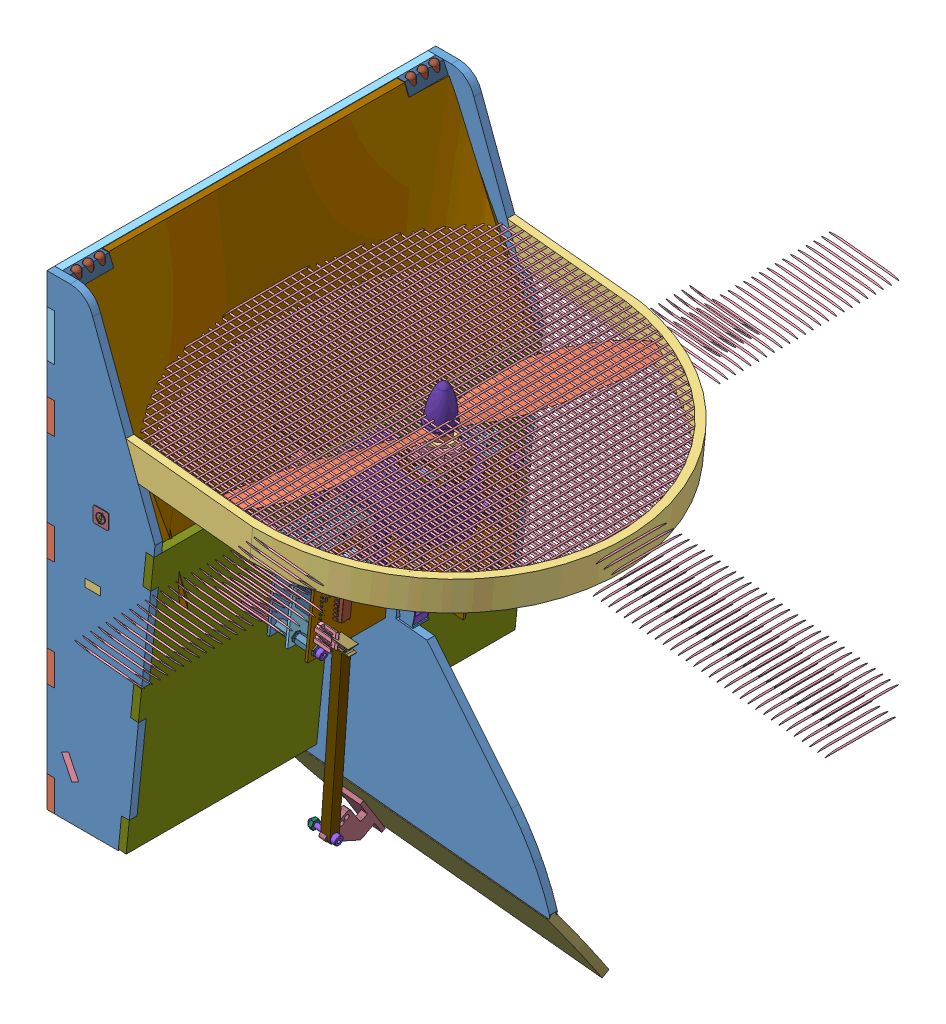
SolidWorks assembly AssTotaleSimu7, configuration Défaut. Lengths in mm. (continued)
Components (placement in the parent): (continued)
- AssStructSimu-1: AssStructSimu [Défaut] at (-125.7658 -1.8483 624.6548) x (1 0 0) z (0 0 -1) size (253.25 324.59 251.6) (continued)
  - AssProtec-1: AssProtec [Défaut] at (86.6746 190.4649 284.6351) x (0 0 -1) z (0.101852 -0.9948 0) size (250 237.46 20) (continued)
    - AssGrillage-2: AssGrillage [Défaut] at (339.6086 -132.5428 241.6839) x (0 0 1) z (-1 0 0) size (2.02 237.05 250) (continued)
      - barreau-208: barreau [Défaut] at (-0.1839 -1.5314 233.7823) x (0.998922 0 0.04641) z (0 1 0) size (1 1 400)
      - barreau-209: barreau [Défaut] at (-0.1839 -1.5314 228.7823) x (0.998922 0 0.04641) z (0 1 0) size (1 1 400)
      - barreau-210: barreau [Défaut] at (-0.1839 -1.5314 223.7823) x (0.998922 0 0.04641) z (0 1 0) size (1 1 400)
      - barreau-211: barreau [Défaut] at (-0.1839 -1.5314 218.7823) x (0.998922 0 0.04641) z (0 1 0) size (1 1 400)
      - barreau-212: barreau [Défaut] at (-0.1839 -1.5314 213.7823) x (0.998922 0 0.04641) z (0 1 0) size (1 1 400)
      - barreau-213: barreau [Défaut] at (-0.1839 -1.5314 208.7823) x (0.998922 0 0.04641) z (0 1 0) size (1 1 400)
      - barreau-214: barreau [Défaut] at (-0.1839 -1.5314 203.7823) x (0.998922 0 0.04641) z (0 1 0) size (1 1 400)
  - AssCarte-1: AssCarte [Défaut] at (38.0121 147.1029 290.772) x (-0.101852 0.9948 0) z (0.9948 0.101852 0) size (66.52 130.57 98.72)
    - carte_onduleur_v3-1: carte_onduleur_v3 [Défaut] at (-131.8199 12.0892 20.7912) size (66.52 130.57 82.34)
      - Layer_1-1: Layer_1 [Défaut] at origin size (60 130 1.61)
      - BTN-1: BTN [Défaut] at (-25.5 7.4 0.803) x (0 -1 0) z (0 0 1) size (6.76 3.64 4.37)
        - Open CASCADE STEP translator 6.8 1.2.1-1: Open CASCADE STEP translator 6.8 1.2.1 [Défaut] at origin size (6.76 3.64 4.37)
          - Body_1-1: Body_1 [Défaut] at (-0.5 -2 0) size (6.76 3.64 4.37)
            - =_[0_1_1_3]-1: =_[0_1_1_3] [Défaut] at origin size (6 3.64 4.37)
            - =_[0_1_1_4]-1: =_[0_1_1_4] [Défaut] at origin size (0.38 1 0.67)
            - =_[0_1_1_5]-1: =_[0_1_1_5] [Défaut] at origin size (0.38 1 0.67)
      - CON_IO1-1: CON_IO1 [Défaut] at (-11.3 12.1 0.803) x (0 -1 0) z (0 0 1) size (13 30 57.5)
        - Open CASCADE STEP translator 6.8 1.3.1-1: Open CASCADE STEP translator 6.8 1.3.1 [Défaut] at origin size (13 30 57.5)
          - Body_1_2-1: Body_1_2 [Défaut] at (-3 -15 8) x (0 -1 0) z (-1 0 0) size (30 57.5 13)
            - 1-1: 1 [Défaut] at origin size (30 50 1.61)
            - 10-1: 10 [Défaut] at (-14.395 31.0465 0.803) x (-1 0 0) z (0 0 1) size (5.59 6.35 1.11)
              - =_[0_1_1_4]-1: =_[0_1_1_4] [Défaut] at origin size (5.59 6.35 1.11)
                - 11-1: 11 [Défaut] at (2 3.3 0) x (-1 0 0) z (0 0 1) size (5.59 6.35 1.11)
                  - =_[0_1_1_3]_2-1: =_[0_1_1_3]_2 [Défaut] at origin size (0.44 0.55 0.36)
                  - =_[0_1_1_4]_2-1: =_[0_1_1_4]_2 [Défaut] at origin size (5.59 4.15 0.36)
                  - =_[0_1_1_5]_2-1: =_[0_1_1_5]_2 [Défaut] at origin size (5.35 6.1 1.1)
                  - =_[0_1_1_6]-1: =_[0_1_1_6] [Défaut] at origin size (0.44 0.55 0.36)
                  - =_[0_1_1_7]-1: =_[0_1_1_7] [Défaut] at origin size (0.44 0.55 0.36)
                  - =_[0_1_1_8]-1: =_[0_1_1_8] [Défaut] at origin size (0.44 0.55 0.36)
            - 13-1: 13 [Défaut] at (-12.62 16.6 -0.803) x (-1 0 0) z (0 0 -1) size (5.59 6.35 1.11)
              - =_[0_1_1_13]-1: =_[0_1_1_13] [Défaut] at origin size (5.59 6.35 1.11)
                - 11-1: 11 [Défaut] at (2 3.3 0) x (-1 0 0) z (0 0 1) size (5.59 6.35 1.11)
                  - =_[0_1_1_3]_2-1: =_[0_1_1_3]_2 [Défaut] at origin size (0.44 0.55 0.36)
                  - =_[0_1_1_4]_2-1: =_[0_1_1_4]_2 [Défaut] at origin size (5.59 4.15 0.36)
                  - =_[0_1_1_5]_2-1: =_[0_1_1_5]_2 [Défaut] at origin size (5.35 6.1 1.1)
                  - =_[0_1_1_6]-1: =_[0_1_1_6] [Défaut] at origin size (0.44 0.55 0.36)
                  - =_[0_1_1_7]-1: =_[0_1_1_7] [Défaut] at origin size (0.44 0.55 0.36)
                  - =_[0_1_1_8]-1: =_[0_1_1_8] [Défaut] at origin size (0.44 0.55 0.36)
            - 16-1: 16 [Défaut] at (-4.2 24.2 0.803) x (-1 0 0) z (0 0 1) size (12.8 0.5 13)
              - =_[0_1_1_15]-1: =_[0_1_1_15] [Défaut] at origin size (12.8 0.5 13)
                - 17-1: 17 [Défaut] at (2.7 0 0) x (1 0 0) z (0 -1 0) size (12.8 13 0.5)
            - 19-1: 19 [Défaut] at (-4.1 6.8 0.803) x (-1 0 0) z (0 0 1) size (12.8 0.5 13)
              - =_[0_1_1_18]-1: =_[0_1_1_18] [Défaut] at origin size (12.8 0.5 13)
                - 17-1: 17 [Défaut] at (2.7 0 0) x (1 0 0) z (0 -1 0) size (12.8 13 0.5)
            - 24-1: 24 [Défaut] at (-8.1 16.5 -0.803) x (0 1 0) z (0 0 -1) size (7.75 5.13 1.17)
              - =_[0_1_1_20]-1: =_[0_1_1_20] [Défaut] at origin size (7.75 5.13 1.17)
                - 20-1: 20 [Défaut] at origin size (7.59 5.13 1.07)
                - 21-1: 21 [Défaut] at (-14.478 0 0) x (-1 0 0) z (0 0 1) size (0.76 5.08 1.17)
                - 22-1: 22 [Défaut] at origin size (0.76 5.08 1.17)
            - 35-1: 35 [Défaut] at (-25.3 25.5 0.803) x (0 -1 0) z (0 0 1) size (6.05 5.2 1.7)
              - =_[0_1_1_25]-1: =_[0_1_1_25] [Défaut] at origin size (6.05 5.2 1.7)
                - 25-1: 25 [Défaut] at origin size (4.3 5.2 1.53)
                - 26-1: 26 [Défaut] at origin size (0.88 0.51 1.06)
                - 27-1: 27 [Défaut] at origin size (0.88 0.51 1.06)
                - 28-1: 28 [Défaut] at origin size (0.88 0.51 1.06)
                - 29-1: 29 [Défaut] at origin size (0.88 0.51 1.06)
                - 30-1: 30 [Défaut] at (11.6 -5.08 0) x (-1 0 0) z (0 0 1) size (0.87 0.51 1.06)
                - 31-1: 31 [Défaut] at (11.6 -2.54 0) x (-1 0 0) z (0 0 1) size (0.87 0.51 1.06)
                - 32-1: 32 [Défaut] at (11.6 0 0) x (-1 0 0) z (0 0 1) size (0.87 0.51 1.06)
                - 33-1: 33 [Défaut] at (11.6 2.54 0) x (-1 0 0) z (0 0 1) size (0.87 0.51 1.06)
            - 40-1: 40 [Défaut] at (-27.6 27.2 0.803) size (2.34 1.04 0.5)
              - =_[0_1_1_36]-1: =_[0_1_1_36] [Défaut] at origin size (2.34 1.04 0.5)
                - 36-1: 36 [Défaut] at origin size (2.29 1.04 0.43)
                - 37-1: 37 [Défaut] at (0.3048 0 0) x (-1 0 0) z (0 0 1) size (0.51 1.02 0.5)
                - 38-1: 38 [Défaut] at origin size (0.51 1.02 0.5)
            - 42-1: 42 [Défaut] at (-22.1 21.6 0.803) x (0 1 0) z (0 0 1) size (2.34 1.04 0.5)
              - =_[0_1_1_36]-1: =_[0_1_1_36] [Défaut] at origin size (2.34 1.04 0.5)
                - 36-1: 36 [Défaut] at origin size (2.29 1.04 0.43)
                - 37-1: 37 [Défaut] at (0.3048 0 0) x (-1 0 0) z (0 0 1) size (0.51 1.02 0.5)
                - 38-1: 38 [Défaut] at origin size (0.51 1.02 0.5)
            - 47-1: 47 [Défaut] at (-14.7664 14.5 -0.803) x (-1 0 0) z (0 0 -1) size (2.34 1.04 0.5)
              - =_[0_1_1_42]-1: =_[0_1_1_42] [Défaut] at origin size (2.34 1.04 0.5)
                - 43-1: 43 [Défaut] at origin size (2.29 1.04 0.43)
                - 44-1: 44 [Défaut] at (0.3048 0 0) x (-1 0 0) z (0 0 1) size (0.51 1.02 0.5)
                - 45-1: 45 [Défaut] at origin size (0.51 1.02 0.5)
            - 57-1: 57 [Défaut] at (-15.3 2.7 -0.803) x (0 -1 0) z (0 0 -1) size (10.36 15.24 6.14)
              - =_[0_1_1_47]-1: =_[0_1_1_47] [Défaut] at origin size (10.36 15.24 6.14)
                - 55-1: 55 [Défaut] at (1.8 -1.2 3) x (1 0 0) z (0 1 0) size (10.36 6.14 15.24)
                  - 54-1: 54 [Défaut] at origin size (10.36 6.14 7.62)
                    - 52-1: 52 [Défaut] at origin size (10.36 6.14 2.54)
                      - 48-1: 48 [Défaut] at origin size (8.4 2.54 2.54)
                      - 49-1: 49 [Défaut] at (-0.0461 1.2682 1.27) x (0 0 -1) z (0.999998 -0.002105 0) size (1.95 5.07 7.58)
                    - 52-2: 52 [Défaut] at (0 0 -2.54) size (10.36 6.14 2.54)
                      - 48-1: 48 [Défaut] at origin size (8.4 2.54 2.54)
                      - 49-1: 49 [Défaut] at (-0.0461 1.2682 1.27) x (0 0 -1) z (0.999998 -0.002105 0) size (1.95 5.07 7.58)
                    - 52-3: 52 [Défaut] at (0 0 -5.08) size (10.36 6.14 2.54)
                      - 48-1: 48 [Défaut] at origin size (8.4 2.54 2.54)
                      - 49-1: 49 [Défaut] at (-0.0461 1.2682 1.27) x (0 0 -1) z (0.999998 -0.002105 0) size (1.95 5.07 7.58)
                  - 54-2: 54 [Défaut] at (0 0 -7.62) size (10.36 6.14 7.62)
                    - 52-1: 52 [Défaut] at origin size (10.36 6.14 2.54)
                      - 48-1: 48 [Défaut] at origin size (8.4 2.54 2.54)
                      - 49-1: 49 [Défaut] at (-0.0461 1.2682 1.27) x (0 0 -1) z (0.999998 -0.002105 0) size (1.95 5.07 7.58)
                    - 52-2: 52 [Défaut] at (0 0 -2.54) size (10.36 6.14 2.54)
                      - 48-1: 48 [Défaut] at origin size (8.4 2.54 2.54)
                      - 49-1: 49 [Défaut] at (-0.0461 1.2682 1.27) x (0 0 -1) z (0.999998 -0.002105 0) size (1.95 5.07 7.58)
                    - 52-3: 52 [Défaut] at (0 0 -5.08) size (10.36 6.14 2.54)
                      - 48-1: 48 [Défaut] at origin size (8.4 2.54 2.54)
                      - 49-1: 49 [Défaut] at (-0.0461 1.2682 1.27) x (0 0 -1) z (0.999998 -0.002105 0) size (1.95 5.07 7.58)
            - 59-1: 59 [Défaut] at (-26.5 31 0.803) x (0 -1 0) z (0 0 1) size (2.34 1.04 0.5)
              - =_[0_1_1_42]-1: =_[0_1_1_42] [Défaut] at origin size (2.34 1.04 0.5)
                - 43-1: 43 [Défaut] at origin size (2.29 1.04 0.43)
                - 44-1: 44 [Défaut] at (0.3048 0 0) x (-1 0 0) z (0 0 1) size (0.51 1.02 0.5)
                - 45-1: 45 [Défaut] at origin size (0.51 1.02 0.5)
            - 61-1: 61 [Défaut] at (-21.6 17.8 0.803) x (-1 0 0) z (0 0 1) size (2.34 1.04 0.5)
              - =_[0_1_1_42]-1: =_[0_1_1_42] [Défaut] at origin size (2.34 1.04 0.5)
                - 43-1: 43 [Défaut] at origin size (2.29 1.04 0.43)
                - 44-1: 44 [Défaut] at (0.3048 0 0) x (-1 0 0) z (0 0 1) size (0.51 1.02 0.5)
                - 45-1: 45 [Défaut] at origin size (0.51 1.02 0.5)
            - 74-1: 74 [Défaut] at (-4.9 41.8 0.803) x (0 -1 0) z (0 0 1) size (6 4.9 1.75)
              - =_[0_1_1_56]-1: =_[0_1_1_56] [Défaut] at origin size (6 4.9 1.75)
                - 72-1: 72 [Défaut] at origin size (6 4.9 1.75)
                  - =_[0_1_1_2]-1: =_[0_1_1_2] [Défaut] at origin size (3.9 4.9 1.57)
                  - =_[0_1_1_3]-1: =_[0_1_1_3] [Défaut] at origin size (6 4.22 1)
                    - =_[0_1_1_60]-1: =_[0_1_1_60] [Défaut] at origin size (1.05 0.41 1)
                    - =_[0_1_1_61]-1: =_[0_1_1_61] [Défaut] at origin size (1.05 0.41 1)
                    - =_[0_1_1_62]-1: =_[0_1_1_62] [Défaut] at origin size (1.05 0.41 1)
                    - =_[0_1_1_63]-1: =_[0_1_1_63] [Défaut] at origin size (1.05 0.41 1)
                    - =_[0_1_1_64]-1: =_[0_1_1_64] [Défaut] at origin size (1.05 0.41 1)
                    - =_[0_1_1_65]-1: =_[0_1_1_65] [Défaut] at origin size (1.05 0.41 1)
                    - =_[0_1_1_66]-1: =_[0_1_1_66] [Défaut] at origin size (1.05 0.41 1)
                    - =_[0_1_1_67]-1: =_[0_1_1_67] [Défaut] at origin size (1.05 0.41 1)
            - 76-1: 76 [Défaut] at (-8.5 40.5664 0.803) x (0 1 0) z (0 0 1) size (2.34 1.04 0.5)
              - =_[0_1_1_42]-1: =_[0_1_1_42] [Défaut] at origin size (2.34 1.04 0.5)
                - 43-1: 43 [Défaut] at origin size (2.29 1.04 0.43)
                - 44-1: 44 [Défaut] at (0.3048 0 0) x (-1 0 0) z (0 0 1) size (0.51 1.02 0.5)
                - 45-1: 45 [Défaut] at origin size (0.51 1.02 0.5)
            - 78-1: 78 [Défaut] at (-5.9 46.4 0.803) x (-1 0 0) z (0 0 1) size (2.34 1.04 0.5)
              - =_[0_1_1_42]-1: =_[0_1_1_42] [Défaut] at origin size (2.34 1.04 0.5)
                - 43-1: 43 [Défaut] at origin size (2.29 1.04 0.43)
                - 44-1: 44 [Défaut] at (0.3048 0 0) x (-1 0 0) z (0 0 1) size (0.51 1.02 0.5)
                - 45-1: 45 [Défaut] at origin size (0.51 1.02 0.5)
            - 80-1: 80 [Défaut] at (-7 48.1 0.803) size (2.34 1.04 0.5)
              - =_[0_1_1_42]-1: =_[0_1_1_42] [Défaut] at origin size (2.34 1.04 0.5)
                - 43-1: 43 [Défaut] at origin size (2.29 1.04 0.43)
                - 44-1: 44 [Défaut] at (0.3048 0 0) x (-1 0 0) z (0 0 1) size (0.51 1.02 0.5)
                - 45-1: 45 [Défaut] at origin size (0.51 1.02 0.5)
            - 82-1: 82 [Défaut] at (-6 37.1 0.803) size (2.34 1.04 0.5)
              - =_[0_1_1_42]-1: =_[0_1_1_42] [Défaut] at origin size (2.34 1.04 0.5)
                - 43-1: 43 [Défaut] at origin size (2.29 1.04 0.43)
                - 44-1: 44 [Défaut] at (0.3048 0 0) x (-1 0 0) z (0 0 1) size (0.51 1.02 0.5)
                - 45-1: 45 [Défaut] at origin size (0.51 1.02 0.5)
      - CON_IO2-1: CON_IO2 [Défaut] at (-11.3 -2.7 0.803) x (0 -1 0) z (0 0 1) size (13 30 57.5)
        - Open CASCADE STEP translator 6.8 1.4.1-1: Open CASCADE STEP translator 6.8 1.4.1 [Défaut] at origin size (13 30 57.5)
          - Body_1_2-1: Body_1_2 [Défaut] at (-3 -15 8) x (0 -1 0) z (-1 0 0) size (30 57.5 13)
            - 1-1: 1 [Défaut] at origin size (30 50 1.61)
            - 10-1: 10 [Défaut] at (-14.395 31.0465 0.803) x (-1 0 0) z (0 0 1) size (5.59 6.35 1.11)
              - =_[0_1_1_4]-1: =_[0_1_1_4] [Défaut] at origin size (5.59 6.35 1.11)
                - 11-1: 11 [Défaut] at (2 3.3 0) x (-1 0 0) z (0 0 1) size (5.59 6.35 1.11)
                  - =_[0_1_1_3]_2-1: =_[0_1_1_3]_2 [Défaut] at origin size (0.44 0.55 0.36)
                  - =_[0_1_1_4]_2-1: =_[0_1_1_4]_2 [Défaut] at origin size (5.59 4.15 0.36)
                  - =_[0_1_1_5]_2-1: =_[0_1_1_5]_2 [Défaut] at origin size (5.35 6.1 1.1)
                  - =_[0_1_1_6]-1: =_[0_1_1_6] [Défaut] at origin size (0.44 0.55 0.36)
                  - =_[0_1_1_7]-1: =_[0_1_1_7] [Défaut] at origin size (0.44 0.55 0.36)
                  - =_[0_1_1_8]-1: =_[0_1_1_8] [Défaut] at origin size (0.44 0.55 0.36)
            - 13-1: 13 [Défaut] at (-12.62 16.6 -0.803) x (-1 0 0) z (0 0 -1) size (5.59 6.35 1.11)
              - =_[0_1_1_13]-1: =_[0_1_1_13] [Défaut] at origin size (5.59 6.35 1.11)
                - 11-1: 11 [Défaut] at (2 3.3 0) x (-1 0 0) z (0 0 1) size (5.59 6.35 1.11)
                  - =_[0_1_1_3]_2-1: =_[0_1_1_3]_2 [Défaut] at origin size (0.44 0.55 0.36)
                  - =_[0_1_1_4]_2-1: =_[0_1_1_4]_2 [Défaut] at origin size (5.59 4.15 0.36)
                  - =_[0_1_1_5]_2-1: =_[0_1_1_5]_2 [Défaut] at origin size (5.35 6.1 1.1)
                  - =_[0_1_1_6]-1: =_[0_1_1_6] [Défaut] at origin size (0.44 0.55 0.36)
                  - =_[0_1_1_7]-1: =_[0_1_1_7] [Défaut] at origin size (0.44 0.55 0.36)
                  - =_[0_1_1_8]-1: =_[0_1_1_8] [Défaut] at origin size (0.44 0.55 0.36)
            - 16-1: 16 [Défaut] at (-4.2 24.2 0.803) x (-1 0 0) z (0 0 1) size (12.8 0.5 13)
              - =_[0_1_1_15]-1: =_[0_1_1_15] [Défaut] at origin size (12.8 0.5 13)
                - 17-1: 17 [Défaut] at (2.7 0 0) x (1 0 0) z (0 -1 0) size (12.8 13 0.5)
            - 19-1: 19 [Défaut] at (-4.1 6.8 0.803) x (-1 0 0) z (0 0 1) size (12.8 0.5 13)
              - =_[0_1_1_18]-1: =_[0_1_1_18] [Défaut] at origin size (12.8 0.5 13)
                - 17-1: 17 [Défaut] at (2.7 0 0) x (1 0 0) z (0 -1 0) size (12.8 13 0.5)
            - 24-1: 24 [Défaut] at (-8.1 16.5 -0.803) x (0 1 0) z (0 0 -1) size (7.75 5.13 1.17)
              - =_[0_1_1_20]-1: =_[0_1_1_20] [Défaut] at origin size (7.75 5.13 1.17)
                - 20-1: 20 [Défaut] at origin size (7.59 5.13 1.07)
                - 21-1: 21 [Défaut] at (-14.478 0 0) x (-1 0 0) z (0 0 1) size (0.76 5.08 1.17)
                - 22-1: 22 [Défaut] at origin size (0.76 5.08 1.17)
            - 35-1: 35 [Défaut] at (-25.3 25.5 0.803) x (0 -1 0) z (0 0 1) size (6.05 5.2 1.7)
              - =_[0_1_1_25]-1: =_[0_1_1_25] [Défaut] at origin size (6.05 5.2 1.7)
                - 25-1: 25 [Défaut] at origin size (4.3 5.2 1.53)
                - 26-1: 26 [Défaut] at origin size (0.88 0.51 1.06)
                - 27-1: 27 [Défaut] at origin size (0.88 0.51 1.06)
                - 28-1: 28 [Défaut] at origin size (0.88 0.51 1.06)
                - 29-1: 29 [Défaut] at origin size (0.88 0.51 1.06)
                - 30-1: 30 [Défaut] at (11.6 -5.08 0) x (-1 0 0) z (0 0 1) size (0.87 0.51 1.06)
                - 31-1: 31 [Défaut] at (11.6 -2.54 0) x (-1 0 0) z (0 0 1) size (0.87 0.51 1.06)
                - 32-1: 32 [Défaut] at (11.6 0 0) x (-1 0 0) z (0 0 1) size (0.87 0.51 1.06)
                - 33-1: 33 [Défaut] at (11.6 2.54 0) x (-1 0 0) z (0 0 1) size (0.87 0.51 1.06)
            - 40-1: 40 [Défaut] at (-27.6 27.2 0.803) size (2.34 1.04 0.5)
              - =_[0_1_1_36]-1: =_[0_1_1_36] [Défaut] at origin size (2.34 1.04 0.5)
                - 36-1: 36 [Défaut] at origin size (2.29 1.04 0.43)
                - 37-1: 37 [Défaut] at (0.3048 0 0) x (-1 0 0) z (0 0 1) size (0.51 1.02 0.5)
                - 38-1: 38 [Défaut] at origin size (0.51 1.02 0.5)
            - 42-1: 42 [Défaut] at (-22.1 21.6 0.803) x (0 1 0) z (0 0 1) size (2.34 1.04 0.5)
              - =_[0_1_1_36]-1: =_[0_1_1_36] [Défaut] at origin size (2.34 1.04 0.5)
                - 36-1: 36 [Défaut] at origin size (2.29 1.04 0.43)
                - 37-1: 37 [Défaut] at (0.3048 0 0) x (-1 0 0) z (0 0 1) size (0.51 1.02 0.5)
                - 38-1: 38 [Défaut] at origin size (0.51 1.02 0.5)
            - 47-1: 47 [Défaut] at (-14.7664 14.5 -0.803) x (-1 0 0) z (0 0 -1) size (2.34 1.04 0.5)
              - =_[0_1_1_42]-1: =_[0_1_1_42] [Défaut] at origin size (2.34 1.04 0.5)
                - 43-1: 43 [Défaut] at origin size (2.29 1.04 0.43)
                - 44-1: 44 [Défaut] at (0.3048 0 0) x (-1 0 0) z (0 0 1) size (0.51 1.02 0.5)
                - 45-1: 45 [Défaut] at origin size (0.51 1.02 0.5)
            - 57-1: 57 [Défaut] at (-15.3 2.7 -0.803) x (0 -1 0) z (0 0 -1) size (10.36 15.24 6.14)
              - =_[0_1_1_47]-1: =_[0_1_1_47] [Défaut] at origin size (10.36 15.24 6.14)
                - 55-1: 55 [Défaut] at (1.8 -1.2 3) x (1 0 0) z (0 1 0) size (10.36 6.14 15.24)
                  - 54-1: 54 [Défaut] at origin size (10.36 6.14 7.62)
                    - 52-1: 52 [Défaut] at origin size (10.36 6.14 2.54)
                      - 48-1: 48 [Défaut] at origin size (8.4 2.54 2.54)
                      - 49-1: 49 [Défaut] at (-0.0461 1.2682 1.27) x (0 0 -1) z (0.999998 -0.002105 0) size (1.95 5.07 7.58)
                    - 52-2: 52 [Défaut] at (0 0 -2.54) size (10.36 6.14 2.54)
                      - 48-1: 48 [Défaut] at origin size (8.4 2.54 2.54)
                      - 49-1: 49 [Défaut] at (-0.0461 1.2682 1.27) x (0 0 -1) z (0.999998 -0.002105 0) size (1.95 5.07 7.58)
                    - 52-3: 52 [Défaut] at (0 0 -5.08) size (10.36 6.14 2.54)
                      - 48-1: 48 [Défaut] at origin size (8.4 2.54 2.54)
                      - 49-1: 49 [Défaut] at (-0.0461 1.2682 1.27) x (0 0 -1) z (0.999998 -0.002105 0) size (1.95 5.07 7.58)
                  - 54-2: 54 [Défaut] at (0 0 -7.62) size (10.36 6.14 7.62)
                    - 52-1: 52 [Défaut] at origin size (10.36 6.14 2.54)
                      - 48-1: 48 [Défaut] at origin size (8.4 2.54 2.54)
                      - 49-1: 49 [Défaut] at (-0.0461 1.2682 1.27) x (0 0 -1) z (0.999998 -0.002105 0) size (1.95 5.07 7.58)
                    - 52-2: 52 [Défaut] at (0 0 -2.54) size (10.36 6.14 2.54)
                      - 48-1: 48 [Défaut] at origin size (8.4 2.54 2.54)
                      - 49-1: 49 [Défaut] at (-0.0461 1.2682 1.27) x (0 0 -1) z (0.999998 -0.002105 0) size (1.95 5.07 7.58)
                    - 52-3: 52 [Défaut] at (0 0 -5.08) size (10.36 6.14 2.54)
                      - 48-1: 48 [Défaut] at origin size (8.4 2.54 2.54)
                      - 49-1: 49 [Défaut] at (-0.0461 1.2682 1.27) x (0 0 -1) z (0.999998 -0.002105 0) size (1.95 5.07 7.58)
            - 59-1: 59 [Défaut] at (-26.5 31 0.803) x (0 -1 0) z (0 0 1) size (2.34 1.04 0.5)
              - =_[0_1_1_42]-1: =_[0_1_1_42] [Défaut] at origin size (2.34 1.04 0.5)
                - 43-1: 43 [Défaut] at origin size (2.29 1.04 0.43)
                - 44-1: 44 [Défaut] at (0.3048 0 0) x (-1 0 0) z (0 0 1) size (0.51 1.02 0.5)
                - 45-1: 45 [Défaut] at origin size (0.51 1.02 0.5)
            - 61-1: 61 [Défaut] at (-21.6 17.8 0.803) x (-1 0 0) z (0 0 1) size (2.34 1.04 0.5)
              - =_[0_1_1_42]-1: =_[0_1_1_42] [Défaut] at origin size (2.34 1.04 0.5)
                - 43-1: 43 [Défaut] at origin size (2.29 1.04 0.43)
                - 44-1: 44 [Défaut] at (0.3048 0 0) x (-1 0 0) z (0 0 1) size (0.51 1.02 0.5)
                - 45-1: 45 [Défaut] at origin size (0.51 1.02 0.5)
            - 74-1: 74 [Défaut] at (-4.9 41.8 0.803) x (0 -1 0) z (0 0 1) size (6 4.9 1.75)
              - =_[0_1_1_56]-1: =_[0_1_1_56] [Défaut] at origin size (6 4.9 1.75)
                - 72-1: 72 [Défaut] at origin size (6 4.9 1.75)
                  - =_[0_1_1_2]-1: =_[0_1_1_2] [Défaut] at origin size (3.9 4.9 1.57)
                  - =_[0_1_1_3]-1: =_[0_1_1_3] [Défaut] at origin size (6 4.22 1)
                    - =_[0_1_1_60]-1: =_[0_1_1_60] [Défaut] at origin size (1.05 0.41 1)
                    - =_[0_1_1_61]-1: =_[0_1_1_61] [Défaut] at origin size (1.05 0.41 1)
                    - =_[0_1_1_62]-1: =_[0_1_1_62] [Défaut] at origin size (1.05 0.41 1)
                    - =_[0_1_1_63]-1: =_[0_1_1_63] [Défaut] at origin size (1.05 0.41 1)
                    - =_[0_1_1_64]-1: =_[0_1_1_64] [Défaut] at origin size (1.05 0.41 1)
                    - =_[0_1_1_65]-1: =_[0_1_1_65] [Défaut] at origin size (1.05 0.41 1)
                    - =_[0_1_1_66]-1: =_[0_1_1_66] [Défaut] at origin size (1.05 0.41 1)
                    - =_[0_1_1_67]-1: =_[0_1_1_67] [Défaut] at origin size (1.05 0.41 1)
            - 76-1: 76 [Défaut] at (-8.5 40.5664 0.803) x (0 1 0) z (0 0 1) size (2.34 1.04 0.5)
              - =_[0_1_1_42]-1: =_[0_1_1_42] [Défaut] at origin size (2.34 1.04 0.5)
                - 43-1: 43 [Défaut] at origin size (2.29 1.04 0.43)
                - 44-1: 44 [Défaut] at (0.3048 0 0) x (-1 0 0) z (0 0 1) size (0.51 1.02 0.5)
                - 45-1: 45 [Défaut] at origin size (0.51 1.02 0.5)
            - 78-1: 78 [Défaut] at (-5.9 46.4 0.803) x (-1 0 0) z (0 0 1) size (2.34 1.04 0.5)
              - =_[0_1_1_42]-1: =_[0_1_1_42] [Défaut] at origin size (2.34 1.04 0.5)
                - 43-1: 43 [Défaut] at origin size (2.29 1.04 0.43)
                - 44-1: 44 [Défaut] at (0.3048 0 0) x (-1 0 0) z (0 0 1) size (0.51 1.02 0.5)
                - 45-1: 45 [Défaut] at origin size (0.51 1.02 0.5)
            - 80-1: 80 [Défaut] at (-7 48.1 0.803) size (2.34 1.04 0.5)
              - =_[0_1_1_42]-1: =_[0_1_1_42] [Défaut] at origin size (2.34 1.04 0.5)
                - 43-1: 43 [Défaut] at origin size (2.29 1.04 0.43)
                - 44-1: 44 [Défaut] at (0.3048 0 0) x (-1 0 0) z (0 0 1) size (0.51 1.02 0.5)
                - 45-1: 45 [Défaut] at origin size (0.51 1.02 0.5)
            - 82-1: 82 [Défaut] at (-6 37.1 0.803) size (2.34 1.04 0.5)
              - =_[0_1_1_42]-1: =_[0_1_1_42] [Défaut] at origin size (2.34 1.04 0.5)
                - 43-1: 43 [Défaut] at origin size (2.29 1.04 0.43)
                - 44-1: 44 [Défaut] at (0.3048 0 0) x (-1 0 0) z (0 0 1) size (0.51 1.02 0.5)
                - 45-1: 45 [Défaut] at origin size (0.51 1.02 0.5)
      - CON_IO3-1: CON_IO3 [Défaut] at (-11.3 -17.7 0.803) x (0 -1 0) z (0 0 1) size (13 30 57.5)
        - Open CASCADE STEP translator 6.8 1.5.1-1: Open CASCADE STEP translator 6.8 1.5.1 [Défaut] at origin size (13 30 57.5)
          - Body_1_2-1: Body_1_2 [Défaut] at (-3 -15 8) x (0 -1 0) z (-1 0 0) size (30 57.5 13)
            - 1-1: 1 [Défaut] at origin size (30 50 1.61)
            - 10-1: 10 [Défaut] at (-14.395 31.0465 0.803) x (-1 0 0) z (0 0 1) size (5.59 6.35 1.11)
              - =_[0_1_1_4]-1: =_[0_1_1_4] [Défaut] at origin size (5.59 6.35 1.11)
                - 11-1: 11 [Défaut] at (2 3.3 0) x (-1 0 0) z (0 0 1) size (5.59 6.35 1.11)
                  - =_[0_1_1_3]_2-1: =_[0_1_1_3]_2 [Défaut] at origin size (0.44 0.55 0.36)
                  - =_[0_1_1_4]_2-1: =_[0_1_1_4]_2 [Défaut] at origin size (5.59 4.15 0.36)
                  - =_[0_1_1_5]_2-1: =_[0_1_1_5]_2 [Défaut] at origin size (5.35 6.1 1.1)
                  - =_[0_1_1_6]-1: =_[0_1_1_6] [Défaut] at origin size (0.44 0.55 0.36)
                  - =_[0_1_1_7]-1: =_[0_1_1_7] [Défaut] at origin size (0.44 0.55 0.36)
                  - =_[0_1_1_8]-1: =_[0_1_1_8] [Défaut] at origin size (0.44 0.55 0.36)
            - 13-1: 13 [Défaut] at (-12.62 16.6 -0.803) x (-1 0 0) z (0 0 -1) size (5.59 6.35 1.11)
              - =_[0_1_1_13]-1: =_[0_1_1_13] [Défaut] at origin size (5.59 6.35 1.11)
                - 11-1: 11 [Défaut] at (2 3.3 0) x (-1 0 0) z (0 0 1) size (5.59 6.35 1.11)
                  - =_[0_1_1_3]_2-1: =_[0_1_1_3]_2 [Défaut] at origin size (0.44 0.55 0.36)
                  - =_[0_1_1_4]_2-1: =_[0_1_1_4]_2 [Défaut] at origin size (5.59 4.15 0.36)
                  - =_[0_1_1_5]_2-1: =_[0_1_1_5]_2 [Défaut] at origin size (5.35 6.1 1.1)
                  - =_[0_1_1_6]-1: =_[0_1_1_6] [Défaut] at origin size (0.44 0.55 0.36)
                  - =_[0_1_1_7]-1: =_[0_1_1_7] [Défaut] at origin size (0.44 0.55 0.36)
                  - =_[0_1_1_8]-1: =_[0_1_1_8] [Défaut] at origin size (0.44 0.55 0.36)
            - 16-1: 16 [Défaut] at (-4.2 24.2 0.803) x (-1 0 0) z (0 0 1) size (12.8 0.5 13)
              - =_[0_1_1_15]-1: =_[0_1_1_15] [Défaut] at origin size (12.8 0.5 13)
                - 17-1: 17 [Défaut] at (2.7 0 0) x (1 0 0) z (0 -1 0) size (12.8 13 0.5)
            - 19-1: 19 [Défaut] at (-4.1 6.8 0.803) x (-1 0 0) z (0 0 1) size (12.8 0.5 13)
              - =_[0_1_1_18]-1: =_[0_1_1_18] [Défaut] at origin size (12.8 0.5 13)
                - 17-1: 17 [Défaut] at (2.7 0 0) x (1 0 0) z (0 -1 0) size (12.8 13 0.5)
            - 24-1: 24 [Défaut] at (-8.1 16.5 -0.803) x (0 1 0) z (0 0 -1) size (7.75 5.13 1.17)
              - =_[0_1_1_20]-1: =_[0_1_1_20] [Défaut] at origin size (7.75 5.13 1.17)
                - 20-1: 20 [Défaut] at origin size (7.59 5.13 1.07)
                - 21-1: 21 [Défaut] at (-14.478 0 0) x (-1 0 0) z (0 0 1) size (0.76 5.08 1.17)
                - 22-1: 22 [Défaut] at origin size (0.76 5.08 1.17)
            - 35-1: 35 [Défaut] at (-25.3 25.5 0.803) x (0 -1 0) z (0 0 1) size (6.05 5.2 1.7)
              - =_[0_1_1_25]-1: =_[0_1_1_25] [Défaut] at origin size (6.05 5.2 1.7)
                - 25-1: 25 [Défaut] at origin size (4.3 5.2 1.53)
                - 26-1: 26 [Défaut] at origin size (0.88 0.51 1.06)
                - 27-1: 27 [Défaut] at origin size (0.88 0.51 1.06)
                - 28-1: 28 [Défaut] at origin size (0.88 0.51 1.06)
                - 29-1: 29 [Défaut] at origin size (0.88 0.51 1.06)
                - 30-1: 30 [Défaut] at (11.6 -5.08 0) x (-1 0 0) z (0 0 1) size (0.87 0.51 1.06)
                - 31-1: 31 [Défaut] at (11.6 -2.54 0) x (-1 0 0) z (0 0 1) size (0.87 0.51 1.06)
                - 32-1: 32 [Défaut] at (11.6 0 0) x (-1 0 0) z (0 0 1) size (0.87 0.51 1.06)
                - 33-1: 33 [Défaut] at (11.6 2.54 0) x (-1 0 0) z (0 0 1) size (0.87 0.51 1.06)
            - 40-1: 40 [Défaut] at (-27.6 27.2 0.803) size (2.34 1.04 0.5)
              - =_[0_1_1_36]-1: =_[0_1_1_36] [Défaut] at origin size (2.34 1.04 0.5)
                - 36-1: 36 [Défaut] at origin size (2.29 1.04 0.43)
                - 37-1: 37 [Défaut] at (0.3048 0 0) x (-1 0 0) z (0 0 1) size (0.51 1.02 0.5)
                - 38-1: 38 [Défaut] at origin size (0.51 1.02 0.5)
            - 42-1: 42 [Défaut] at (-22.1 21.6 0.803) x (0 1 0) z (0 0 1) size (2.34 1.04 0.5)
              - =_[0_1_1_36]-1: =_[0_1_1_36] [Défaut] at origin size (2.34 1.04 0.5)
                - 36-1: 36 [Défaut] at origin size (2.29 1.04 0.43)
                - 37-1: 37 [Défaut] at (0.3048 0 0) x (-1 0 0) z (0 0 1) size (0.51 1.02 0.5)
                - 38-1: 38 [Défaut] at origin size (0.51 1.02 0.5)
            - 47-1: 47 [Défaut] at (-14.7664 14.5 -0.803) x (-1 0 0) z (0 0 -1) size (2.34 1.04 0.5)
              - =_[0_1_1_42]-1: =_[0_1_1_42] [Défaut] at origin size (2.34 1.04 0.5)
                - 43-1: 43 [Défaut] at origin size (2.29 1.04 0.43)
                - 44-1: 44 [Défaut] at (0.3048 0 0) x (-1 0 0) z (0 0 1) size (0.51 1.02 0.5)
                - 45-1: 45 [Défaut] at origin size (0.51 1.02 0.5)
            - 57-1: 57 [Défaut] at (-15.3 2.7 -0.803) x (0 -1 0) z (0 0 -1) size (10.36 15.24 6.14)
              - =_[0_1_1_47]-1: =_[0_1_1_47] [Défaut] at origin size (10.36 15.24 6.14)
                - 55-1: 55 [Défaut] at (1.8 -1.2 3) x (1 0 0) z (0 1 0) size (10.36 6.14 15.24)
                  - 54-1: 54 [Défaut] at origin size (10.36 6.14 7.62)
                    - 52-1: 52 [Défaut] at origin size (10.36 6.14 2.54)
                      - 48-1: 48 [Défaut] at origin size (8.4 2.54 2.54)
                      - 49-1: 49 [Défaut] at (-0.0461 1.2682 1.27) x (0 0 -1) z (0.999998 -0.002105 0) size (1.95 5.07 7.58)
                    - 52-2: 52 [Défaut] at (0 0 -2.54) size (10.36 6.14 2.54)
                      - 48-1: 48 [Défaut] at origin size (8.4 2.54 2.54)
                      - 49-1: 49 [Défaut] at (-0.0461 1.2682 1.27) x (0 0 -1) z (0.999998 -0.002105 0) size (1.95 5.07 7.58)
                    - 52-3: 52 [Défaut] at (0 0 -5.08) size (10.36 6.14 2.54)
                      - 48-1: 48 [Défaut] at origin size (8.4 2.54 2.54)
                      - 49-1: 49 [Défaut] at (-0.0461 1.2682 1.27) x (0 0 -1) z (0.999998 -0.002105 0) size (1.95 5.07 7.58)
                  - 54-2: 54 [Défaut] at (0 0 -7.62) size (10.36 6.14 7.62)
                    - 52-1: 52 [Défaut] at origin size (10.36 6.14 2.54)
                      - 48-1: 48 [Défaut] at origin size (8.4 2.54 2.54)
                      - 49-1: 49 [Défaut] at (-0.0461 1.2682 1.27) x (0 0 -1) z (0.999998 -0.002105 0) size (1.95 5.07 7.58)
                    - 52-2: 52 [Défaut] at (0 0 -2.54) size (10.36 6.14 2.54)
                      - 48-1: 48 [Défaut] at origin size (8.4 2.54 2.54)
                      - 49-1: 49 [Défaut] at (-0.0461 1.2682 1.27) x (0 0 -1) z (0.999998 -0.002105 0) size (1.95 5.07 7.58)
                    - 52-3: 52 [Défaut] at (0 0 -5.08) size (10.36 6.14 2.54)
                      - 48-1: 48 [Défaut] at origin size (8.4 2.54 2.54)
                      - 49-1: 49 [Défaut] at (-0.0461 1.2682 1.27) x (0 0 -1) z (0.999998 -0.002105 0) size (1.95 5.07 7.58)
            - 59-1: 59 [Défaut] at (-26.5 31 0.803) x (0 -1 0) z (0 0 1) size (2.34 1.04 0.5)
              - =_[0_1_1_42]-1: =_[0_1_1_42] [Défaut] at origin size (2.34 1.04 0.5)
                - 43-1: 43 [Défaut] at origin size (2.29 1.04 0.43)
                - 44-1: 44 [Défaut] at (0.3048 0 0) x (-1 0 0) z (0 0 1) size (0.51 1.02 0.5)
                - 45-1: 45 [Défaut] at origin size (0.51 1.02 0.5)
            - 61-1: 61 [Défaut] at (-21.6 17.8 0.803) x (-1 0 0) z (0 0 1) size (2.34 1.04 0.5)
              - =_[0_1_1_42]-1: =_[0_1_1_42] [Défaut] at origin size (2.34 1.04 0.5)
                - 43-1: 43 [Défaut] at origin size (2.29 1.04 0.43)
                - 44-1: 44 [Défaut] at (0.3048 0 0) x (-1 0 0) z (0 0 1) size (0.51 1.02 0.5)
                - 45-1: 45 [Défaut] at origin size (0.51 1.02 0.5)
            - 74-1: 74 [Défaut] at (-4.9 41.8 0.803) x (0 -1 0) z (0 0 1) size (6 4.9 1.75)
              - =_[0_1_1_56]-1: =_[0_1_1_56] [Défaut] at origin size (6 4.9 1.75)
                - 72-1: 72 [Défaut] at origin size (6 4.9 1.75)
                  - =_[0_1_1_2]-1: =_[0_1_1_2] [Défaut] at origin size (3.9 4.9 1.57)
                  - =_[0_1_1_3]-1: =_[0_1_1_3] [Défaut] at origin size (6 4.22 1)
                    - =_[0_1_1_60]-1: =_[0_1_1_60] [Défaut] at origin size (1.05 0.41 1)
                    - =_[0_1_1_61]-1: =_[0_1_1_61] [Défaut] at origin size (1.05 0.41 1)
                    - =_[0_1_1_62]-1: =_[0_1_1_62] [Défaut] at origin size (1.05 0.41 1)
                    - =_[0_1_1_63]-1: =_[0_1_1_63] [Défaut] at origin size (1.05 0.41 1)
                    - =_[0_1_1_64]-1: =_[0_1_1_64] [Défaut] at origin size (1.05 0.41 1)
                    - =_[0_1_1_65]-1: =_[0_1_1_65] [Défaut] at origin size (1.05 0.41 1)
                    - =_[0_1_1_66]-1: =_[0_1_1_66] [Défaut] at origin size (1.05 0.41 1)
                    - =_[0_1_1_67]-1: =_[0_1_1_67] [Défaut] at origin size (1.05 0.41 1)
            - 76-1: 76 [Défaut] at (-8.5 40.5664 0.803) x (0 1 0) z (0 0 1) size (2.34 1.04 0.5)
              - =_[0_1_1_42]-1: =_[0_1_1_42] [Défaut] at origin size (2.34 1.04 0.5)
                - 43-1: 43 [Défaut] at origin size (2.29 1.04 0.43)
                - 44-1: 44 [Défaut] at (0.3048 0 0) x (-1 0 0) z (0 0 1) size (0.51 1.02 0.5)
                - 45-1: 45 [Défaut] at origin size (0.51 1.02 0.5)
            - 78-1: 78 [Défaut] at (-5.9 46.4 0.803) x (-1 0 0) z (0 0 1) size (2.34 1.04 0.5)
              - =_[0_1_1_42]-1: =_[0_1_1_42] [Défaut] at origin size (2.34 1.04 0.5)
                - 43-1: 43 [Défaut] at origin size (2.29 1.04 0.43)
                - 44-1: 44 [Défaut] at (0.3048 0 0) x (-1 0 0) z (0 0 1) size (0.51 1.02 0.5)
                - 45-1: 45 [Défaut] at origin size (0.51 1.02 0.5)
            - 80-1: 80 [Défaut] at (-7 48.1 0.803) size (2.34 1.04 0.5)
              - =_[0_1_1_42]-1: =_[0_1_1_42] [Défaut] at origin size (2.34 1.04 0.5)
                - 43-1: 43 [Défaut] at origin size (2.29 1.04 0.43)
                - 44-1: 44 [Défaut] at (0.3048 0 0) x (-1 0 0) z (0 0 1) size (0.51 1.02 0.5)
                - 45-1: 45 [Défaut] at origin size (0.51 1.02 0.5)
            - 82-1: 82 [Défaut] at (-6 37.1 0.803) size (2.34 1.04 0.5)
              - =_[0_1_1_42]-1: =_[0_1_1_42] [Défaut] at origin size (2.34 1.04 0.5)
                - 43-1: 43 [Défaut] at origin size (2.29 1.04 0.43)
                - 44-1: 44 [Défaut] at (0.3048 0 0) x (-1 0 0) z (0 0 1) size (0.51 1.02 0.5)
                - 45-1: 45 [Défaut] at origin size (0.51 1.02 0.5)
      - C1_1-1: C1_1 [Défaut] at (-20.6336 6.4 -0.803) x (1 0 0) z (0 0 -1) size (2.34 1.04 0.5)
        - Open CASCADE STEP translator 6.8 1.6.1-1: Open CASCADE STEP translator 6.8 1.6.1 [Défaut] at origin size (2.34 1.04 0.5)
          - Body_1-1: Body_1 [Défaut] at origin size (2.29 1.04 0.43)
          - Pin_1-1: Pin_1 [Défaut] at (0.3048 0 0) x (-1 0 0) z (0 0 1) size (0.51 1.02 0.5)
          - Pin_2-1: Pin_2 [Défaut] at origin size (0.51 1.02 0.5)
      - C1_2-1: C1_2 [Défaut] at (-24.2 6.4 -0.803) x (1 0 0) z (0 0 -1) size (2.34 1.04 0.5)
        - Open CASCADE STEP translator 6.8 1.6.1-1: Open CASCADE STEP translator 6.8 1.6.1 [Défaut] at origin size (2.34 1.04 0.5)
          - Body_1-1: Body_1 [Défaut] at origin size (2.29 1.04 0.43)
          - Pin_1-1: Pin_1 [Défaut] at (0.3048 0 0) x (-1 0 0) z (0 0 1) size (0.51 1.02 0.5)
          - Pin_2-1: Pin_2 [Défaut] at origin size (0.51 1.02 0.5)
      - C_F-1: C_F [Défaut] at (-16.2432 4.45 -0.803) x (0 -1 0) z (0 0 -1) size (2.34 1.04 0.5)
        - Open CASCADE STEP translator 6.8 1.6.1-1: Open CASCADE STEP translator 6.8 1.6.1 [Défaut] at origin size (2.34 1.04 0.5)
          - Body_1-1: Body_1 [Défaut] at origin size (2.29 1.04 0.43)
          - Pin_1-1: Pin_1 [Défaut] at (0.3048 0 0) x (-1 0 0) z (0 0 1) size (0.51 1.02 0.5)
          - Pin_2-1: Pin_2 [Défaut] at origin size (0.51 1.02 0.5)
      - D_LED_STATE1-1: D_LED_STATE1 [Défaut] at (-6.8906 -21.6 0.803) size (2.34 1.04 0.5)
        - Open CASCADE STEP translator 6.8 1.6.1-1: Open CASCADE STEP translator 6.8 1.6.1 [Défaut] at origin size (2.34 1.04 0.5)
          - Body_1-1: Body_1 [Défaut] at origin size (2.29 1.04 0.43)
          - Pin_1-1: Pin_1 [Défaut] at (0.3048 0 0) x (-1 0 0) z (0 0 1) size (0.51 1.02 0.5)
          - Pin_2-1: Pin_2 [Défaut] at origin size (0.51 1.02 0.5)
      - PICKIT-1: PICKIT [Défaut] at (-24.1 -30.5 0.803) size (15.24 5 14.3)
        - Open CASCADE STEP translator 6.8 1.10.1-1: Open CASCADE STEP translator 6.8 1.10.1 [Défaut] at origin size (15.24 5 14.3)
          - Body_1_2-1: Body_1_2 [Défaut] at (6.3 0 12) size (15.24 5 14.3)
      - C_DEC_CUR-1: C_DEC_CUR [Défaut] at (-8.9496 5.7572 -0.803) x (0 1 0) z (0 0 -1) size (2.34 1.04 0.5)
        - Open CASCADE STEP translator 6.8 1.6.1-1: Open CASCADE STEP translator 6.8 1.6.1 [Défaut] at origin size (2.34 1.04 0.5)
          - Body_1-1: Body_1 [Défaut] at origin size (2.29 1.04 0.43)
          - Pin_1-1: Pin_1 [Défaut] at (0.3048 0 0) x (-1 0 0) z (0 0 1) size (0.51 1.02 0.5)
          - Pin_2-1: Pin_2 [Défaut] at origin size (0.51 1.02 0.5)
      - R_F-1: R_F [Défaut] at (-14.65 4.4432 -0.803) x (0 -1 0) z (0 0 -1) size (2.34 1.04 0.5)
        - Open CASCADE STEP translator 6.8 1.12.1-1: Open CASCADE STEP translator 6.8 1.12.1 [Défaut] at origin size (2.34 1.04 0.5)
          - Body_1_3-1: Body_1_3 [Défaut] at origin size (2.29 1.04 0.43)
          - Pin_1_2-1: Pin_1_2 [Défaut] at (0.3048 0 0) x (-1 0 0) z (0 0 1) size (0.51 1.02 0.5)
          - Pin_2_2-1: Pin_2_2 [Défaut] at origin size (0.51 1.02 0.5)
      - R_GAIN1-1: R_GAIN1 [Défaut] at (-13.95 5.7568 -0.803) x (0 1 0) z (0 0 -1) size (2.34 1.04 0.5)
        - Open CASCADE STEP translator 6.8 1.12.1-1: Open CASCADE STEP translator 6.8 1.12.1 [Défaut] at origin size (2.34 1.04 0.5)
          - Body_1_3-1: Body_1_3 [Défaut] at origin size (2.29 1.04 0.43)
          - Pin_1_2-1: Pin_1_2 [Défaut] at (0.3048 0 0) x (-1 0 0) z (0 0 1) size (0.51 1.02 0.5)
          - Pin_2_2-1: Pin_2_2 [Défaut] at origin size (0.51 1.02 0.5)
      - R_GAIN2-1: R_GAIN2 [Défaut] at (-15.65 7.9176 -0.803) x (0 -1 0) z (0 0 -1) size (2.34 1.04 0.5)
        - Open CASCADE STEP translator 6.8 1.12.1-1: Open CASCADE STEP translator 6.8 1.12.1 [Défaut] at origin size (2.34 1.04 0.5)
          - Body_1_3-1: Body_1_3 [Défaut] at origin size (2.29 1.04 0.43)
          - Pin_1_2-1: Pin_1_2 [Défaut] at (0.3048 0 0) x (-1 0 0) z (0 0 1) size (0.51 1.02 0.5)
          - Pin_2_2-1: Pin_2_2 [Défaut] at origin size (0.51 1.02 0.5)
      - R_LED_STATE1-1: R_LED_STATE1 [Défaut] at (-6.9242 -19.9 0.803) size (2.34 1.04 0.5)
        - Open CASCADE STEP translator 6.8 1.12.1-1: Open CASCADE STEP translator 6.8 1.12.1 [Défaut] at origin size (2.34 1.04 0.5)
          - Body_1_3-1: Body_1_3 [Défaut] at origin size (2.29 1.04 0.43)
          - Pin_1_2-1: Pin_1_2 [Défaut] at (0.3048 0 0) x (-1 0 0) z (0 0 1) size (0.51 1.02 0.5)
          - Pin_2_2-1: Pin_2_2 [Défaut] at origin size (0.51 1.02 0.5)
      - R_RESET1-1: R_RESET1 [Défaut] at (-23 7.9 0.803) size (2.34 1.04 0.5)
        - Open CASCADE STEP translator 6.8 1.12.1-1: Open CASCADE STEP translator 6.8 1.12.1 [Défaut] at origin size (2.34 1.04 0.5)
          - Body_1_3-1: Body_1_3 [Défaut] at origin size (2.29 1.04 0.43)
          - Pin_1_2-1: Pin_1_2 [Défaut] at (0.3048 0 0) x (-1 0 0) z (0 0 1) size (0.51 1.02 0.5)
          - Pin_2_2-1: Pin_2_2 [Défaut] at origin size (0.51 1.02 0.5)
